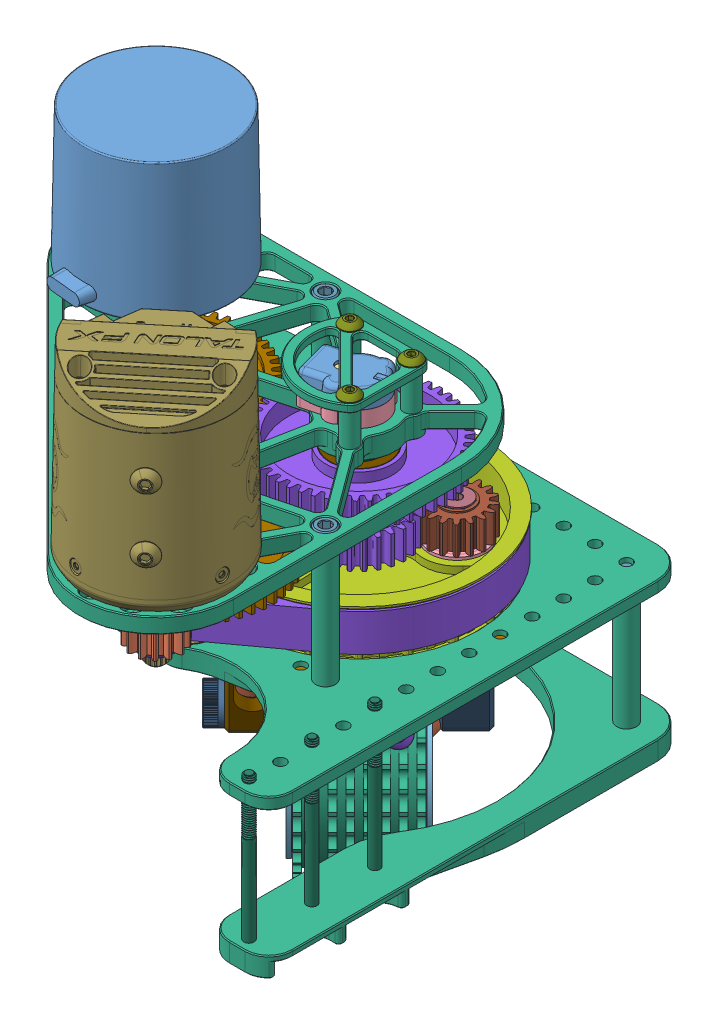
SolidWorks assembly MK4i Swerve Module+KRAKEN, configuration Valor predeterminado. Lengths in mm.
Overall size (247.38 247.71 250.53).
90 component instances, 48 part files, 4 mates.
Components (placement in the parent):
- CANcoder Assembly_MIR1.stp-1: CANcoder Assembly_MIR1.stp [Valor predeterminado] at (-66.675 132.3975 66.675) x (-0.260871 0 -0.965374) z (0 -1 0) size (21.75 26.91 13.51)
  - CANcoder Top Housing_MIR1.stp-1: CANcoder Top Housing_MIR1.stp [Valor predeterminado] at origin size (21.53 26.79 8.94)
  - CANcoder PCA_MIR1.stp-1: CANcoder PCA_MIR1.stp [Valor predeterminado] at (0 0 -22.3055) size (15.93 23.27 3.18)
  - CANcoder Screw_MIR1.stp-1: CANcoder Screw_MIR1.stp [Valor predeterminado] at origin size (4.24 4.24 12.65)
  - CANcoder Bottom Housing_MIR1.stp-1: CANcoder Bottom Housing_MIR1.stp [Valor predeterminado] at origin size (21.75 26.91 6.35)
- MK4 Billet Wheel Assembly_MIR1.stp-1: MK4 Billet Wheel Assembly_MIR1.stp [Valor predeterminado] at (-66.675 50.7435 66.675) x (0.707107 0 -0.707107) z (-0.41117 -0.813559 -0.41117) size (42.28 100.13 100.13)
  - Wheel, SDS, Nitrile Tread, 4in X 1.5in, Bearing Bore_MIR1.stp-1: Wheel, SDS, Nitrile Tread, 4in X 1.5in, Bearing Bore_MIR1.stp [Valor predeterminado] at origin size (42.28 88.9 88.9)
  - Tread, Blue Nitrile 4in X 1.5in_MIR1.stp-1: Tread, Blue Nitrile 4in X 1.5in_MIR1.stp [Valor predeterminado] at origin size (38.1 100.13 100.13)
  - Screw, 10-32 X .75, Button, 91255A269_91255A269_MIR1.stp-1: Screw, 10-32 X .75, Button, 91255A269_91255A269_MIR1.stp [Valor predeterminado] at (-4.826 0 -20.6375) x (0 -0.847203 0.531269) z (1 0 0) size (9.17 9.17 21.62)
  - Screw, 10-32 X .75, Button, 91255A269_91255A269_MIR1.stp-2: Screw, 10-32 X .75, Button, 91255A269_91255A269_MIR1.stp [Valor predeterminado] at (-4.826 -17.8726 -10.3187) x (0 -0.99925 0.038711) z (1 0 0) size (9.17 9.17 21.62)
  - Screw, 10-32 X .75, Button, 91255A269_91255A269_MIR1.stp-3: Screw, 10-32 X .75, Button, 91255A269_91255A269_MIR1.stp [Valor predeterminado] at (-4.826 -17.8726 10.3187) x (0 -0.986188 0.165633) z (1 0 0) size (9.17 9.17 21.62)
  - Screw, 10-32 X .75, Button, 91255A269_91255A269_MIR1.stp-4: Screw, 10-32 X .75, Button, 91255A269_91255A269_MIR1.stp [Valor predeterminado] at (-4.826 0 20.6375) x (0 -0.966455 0.256836) z (1 0 0) size (9.17 9.17 21.62)
  - Screw, 10-32 X .75, Button, 91255A269_91255A269_MIR1.stp-5: Screw, 10-32 X .75, Button, 91255A269_91255A269_MIR1.stp [Valor predeterminado] at (-4.826 17.8726 10.3187) x (0 -0.95104 0.309068) z (1 0 0) size (9.17 9.17 21.62)
  - Screw, 10-32 X .75, Button, 91255A269_91255A269_MIR1.stp-6: Screw, 10-32 X .75, Button, 91255A269_91255A269_MIR1.stp [Valor predeterminado] at (-4.826 17.8726 -10.3187) x (0 -0.947988 0.318305) z (1 0 0) size (9.17 9.17 21.62)
  - Screw, 10-32 X .5, Button, 97763A232_97763A232_MIR1.stp-1: Screw, 10-32 X .5, Button, 97763A232_97763A232_MIR1.stp [Valor predeterminado] at (11.1125 -40.6604 -7.1695) x (-0.785325 0.107503 -0.609678) z (0 0.984808 0.173648) size (9.17 9.17 15.27)
  - Screw, 10-32 X .5, Button, 97763A232_97763A232_MIR1.stp-2: Screw, 10-32 X .5, Button, 97763A232_97763A232_MIR1.stp [Valor predeterminado] at (-11.1125 -40.6604 -7.1695) x (-0.636812 0.133886 -0.759306) z (0 0.984808 0.173648) size (9.17 9.17 15.27)
  - Screw, 10-32 X .5, Button, 97763A232_97763A232_MIR1.stp-3: Screw, 10-32 X .5, Button, 97763A232_97763A232_MIR1.stp [Valor predeterminado] at (-11.1125 -40.6604 7.1695) x (0.726076 -0.119403 -0.677168) z (0 0.984808 -0.173648) size (9.17 9.17 15.27)
  - Screw, 10-32 X .5, Button, 97763A232_97763A232_MIR1.stp-4: Screw, 10-32 X .5, Button, 97763A232_97763A232_MIR1.stp [Valor predeterminado] at (11.1125 -40.6604 7.1695) x (0.841108 -0.09392 -0.53265) z (0 0.984808 -0.173648) size (9.17 9.17 15.27)
  - Screw, 10-32 X .5, Button, 97763A232_97763A232_MIR1.stp-5: Screw, 10-32 X .5, Button, 97763A232_97763A232_MIR1.stp [Valor predeterminado] at (-11.1125 20.6438 35.7562) x (0.804058 -0.514897 0.297276) z (0 -0.5 -0.866025) size (9.17 9.17 15.27)
  - Screw, 10-32 X .5, Button, 97763A232_97763A232_MIR1.stp-6: Screw, 10-32 X .5, Button, 97763A232_97763A232_MIR1.stp [Valor predeterminado] at (11.1125 20.6438 35.7562) x (0.926716 -0.32542 0.187881) z (0 -0.5 -0.866025) size (9.17 9.17 15.27)
  - Screw, 10-32 X .5, Button, 97763A232_97763A232_MIR1.stp-7: Screw, 10-32 X .5, Button, 97763A232_97763A232_MIR1.stp [Valor predeterminado] at (11.1125 20.6438 -35.7562) x (0.200031 0.848523 0.489895) z (0 -0.5 0.866025) size (9.17 9.17 15.27)
  - Screw, 10-32 X .5, Button, 97763A232_97763A232_MIR1.stp-8: Screw, 10-32 X .5, Button, 97763A232_97763A232_MIR1.stp [Valor predeterminado] at (-11.1125 20.6438 -35.7562) x (0.515054 0.74232 0.428579) z (0 -0.5 0.866025) size (9.17 9.17 15.27)
- Screw, 10-32 X .25, Button, 91255A261_91255A261_MIR1.stp-1: Screw, 10-32 X .25, Button, 91255A261_91255A261_MIR1.stp [Valor predeterminado] at (-42.2285 89.5096 114.6539) x (1 0 0) z (0 1 0) size (9.17 9.17 8.92)
- Screw, 10-32 X .25, Button, 91255A261_91255A261_MIR1.stp-2: Screw, 10-32 X .25, Button, 91255A261_91255A261_MIR1.stp [Valor predeterminado] at (-104.7513 89.5096 104.7513) x (0.982082 0 0.188455) z (0 1 0) size (9.17 9.17 8.92)
- Screw, 10-32 X .25, Button, 91255A261_91255A261_MIR1.stp-3: Screw, 10-32 X .25, Button, 91255A261_91255A261_MIR1.stp [Valor predeterminado] at (-114.6539 89.5096 42.2285) x (0.918365 0 0.395734) z (0 1 0) size (9.17 9.17 8.92)
- Screw, 10-32 X .25, Button, 91255A261_91255A261_MIR1.stp-4: Screw, 10-32 X .25, Button, 91255A261_91255A261_MIR1.stp [Valor predeterminado] at (-63.5129 89.5096 12.9199) x (0.8 0 0.6) z (0 1 0) size (9.17 9.17 8.92)
- Screw, 10-32 X .25, Button, 91255A261_91255A261_MIR1.stp-5: Screw, 10-32 X .25, Button, 91255A261_91255A261_MIR1.stp [Valor predeterminado] at (-12.9199 89.5096 63.5129) x (0.63358 0 0.773678) z (0 1 0) size (9.17 9.17 8.92)
- Screw, Shoulder, .375 X 2.5, 5_16-18, 91259A634_91259A634_MIR1.stp-1: Screw, Shoulder, .375 X 2.5, 5_16-18, 91259A634_91259A634_MIR1.stp [Valor predeterminado] at (-93.8403 50.7435 93.8403) x (-0.019195 -0.999631 -0.019195) z (-0.706846 0.027146 -0.706846) size (14.29 82.55 14.29)
- Screw, .25-20 X 1 Socket, 91251A542_91251A542_MIR1.stp-1: Screw, .25-20 X 1 Socket, 91251A542_91251A542_MIR1.stp [Valor predeterminado] at (-102.596 101.6 73.8592) x (0.964329 0 -0.264706) z (0 -1 0) size (9.53 9.53 31.75)
- Screw, .25-20 X 1 Socket, 91251A542_91251A542_MIR1.stp-2: Screw, .25-20 X 1 Socket, 91251A542_91251A542_MIR1.stp [Valor predeterminado] at (-73.8592 101.6 102.596) x (0.982082 0 0.188455) z (0 -1 0) size (9.53 9.53 31.75)
- Screw, .25-20 X .625, 91251A539_91251A539_MIR1.stp-1: Screw, .25-20 X .625, 91251A539_91251A539_MIR1.stp [Valor predeterminado] at (-59.4908 83.2802 30.754) x (1 0 0) z (0 1 0) size (9.53 9.53 22.23)
- Screw, .25-20 X .625, 91251A539_91251A539_MIR1.stp-2: Screw, .25-20 X .625, 91251A539_91251A539_MIR1.stp [Valor predeterminado] at (-30.754 83.2802 59.4908) x (0.982082 0 0.188455) z (0 1 0) size (9.53 9.53 22.23)
- Screw, .25-20 X .625, 91251A539_91251A539_MIR1.stp-3: Screw, .25-20 X .625, 91251A539_91251A539_MIR1.stp [Valor predeterminado] at (-66.675 126.2062 66.675) x (0 0 -1) z (0 -1 0) size (9.53 9.53 22.23)
- Screw, 12-24 X .625, Flat, 91253A282_91253A282_MIR1.stp-1: Screw, 12-24 X .625, Flat, 91253A282_91253A282_MIR1.stp [Valor predeterminado] at (-46.8646 122.8979 46.8646) x (-0.837169 0 0.546944) z (0 -1 0) size (10.72 10.72 15.88)
- Screw, 10-32 X 2.25, 91251A354_91251A354_MIR1.stp-1: Screw, 10-32 X 2.25, 91251A354_91251A354_MIR1.stp [Valor predeterminado] at (-124.5154 92.0115 124.5154) x (-0.750514 0 -0.660855) z (0 1 0) size (7.92 7.92 61.98)
- Screw, 10-32 X 2.25, 91251A354_91251A354_MIR1.stp-2: Screw, 10-32 X 2.25, 91251A354_91251A354_MIR1.stp [Valor predeterminado] at (-32.639 92.0115 114.3) x (-0.612525 0 -0.790452) z (0 1 0) size (7.92 7.92 61.98)
- Screw, 10-32 X 2.25, 91251A354_91251A354_MIR1.stp-3: Screw, 10-32 X 2.25, 91251A354_91251A354_MIR1.stp [Valor predeterminado] at (-114.3 92.0115 32.639) x (-0.427723 0 -0.90391) z (0 1 0) size (7.92 7.92 61.98)
- Screw, 10-32 X 2.25, 91251A354_91251A354_MIR1.stp-4: Screw, 10-32 X 2.25, 91251A354_91251A354_MIR1.stp [Valor predeterminado] at (-12.7 98.4885 12.7) x (0.90391 0 0.427723) z (0 -1 0) size (7.92 7.92 61.98)
- Screw, 8-32 X 2.5, 91251A207_91251A207_MIR1.stp-1: Screw, 8-32 X 2.5, 91251A207_91251A207_MIR1.stp [Valor predeterminado] at (-114.3 102.6795 12.7) x (-0.783238 0 0.621722) z (0 -1 0) size (6.86 6.86 66.17)
- Screw, 8-32 X 2.5, 91251A207_91251A207_MIR1.stp-2: Screw, 8-32 X 2.5, 91251A207_91251A207_MIR1.stp [Valor predeterminado] at (-139.7 102.6795 12.7) x (-0.925243 0 0.379375) z (0 -1 0) size (6.86 6.86 66.17)
- Screw, 8-32 X 2.5, 91251A207_91251A207_MIR1.stp-3: Screw, 8-32 X 2.5, 91251A207_91251A207_MIR1.stp [Valor predeterminado] at (-165.1 102.6795 12.7) x (-0.985271 0 0.170998) z (0 -1 0) size (6.86 6.86 66.17)
- Screw, 8-32 X 2.5, 91251A207_91251A207_MIR1.stp-4: Screw, 8-32 X 2.5, 91251A207_91251A207_MIR1.stp [Valor predeterminado] at (-12.7 102.6795 114.3) x (-0.997902 0 -0.064746) z (0 -1 0) size (6.86 6.86 66.17)
- Screw, 8-32 X 2.5, 91251A207_91251A207_MIR1.stp-5: Screw, 8-32 X 2.5, 91251A207_91251A207_MIR1.stp [Valor predeterminado] at (-12.7 102.6795 139.7) x (-0.953572 0 -0.301166) z (0 -1 0) size (6.86 6.86 66.17)
- Screw, 8-32 X 2.5, 91251A207_91251A207_MIR1.stp-6: Screw, 8-32 X 2.5, 91251A207_91251A207_MIR1.stp [Valor predeterminado] at (-12.7 102.6795 165.1) x (-0.86157 0 -0.507639) z (0 -1 0) size (6.86 6.86 66.17)
- Screw, 8-32 X .875, Button, 91255A166_91255A166_MIR1.stp-1: Screw, 8-32 X .875, Button, 91255A166_91255A166_MIR1.stp [Valor predeterminado] at (-80.9791 172.8661 56.1146) x (1 0 0) z (0 -1 0) size (7.92 7.92 24.45)
- Screw, 8-32 X .875, Button, 91255A166_91255A166_MIR1.stp-2: Screw, 8-32 X .875, Button, 91255A166_91255A166_MIR1.stp [Valor predeterminado] at (-56.1231 172.8661 56.1146) x (0.982082 0 0.188455) z (0 -1 0) size (7.92 7.92 24.45)
- Screw, 8-32 X .875, Button, 91255A166_91255A166_MIR1.stp-3: Screw, 8-32 X .875, Button, 91255A166_91255A166_MIR1.stp [Valor predeterminado] at (-56.1231 172.8661 80.9854) x (0.918365 0 0.395734) z (0 -1 0) size (7.92 7.92 24.45)
- Shim, 8mm ID X 14mm OD X .5mm Thick, 98055A115_98055A115_MIR1.stp-1: Shim, 8mm ID X 14mm OD X .5mm Thick, 98055A115_98055A115_MIR1.stp [Valor predeterminado] at (-46.8646 73.9775 46.8646) x (0.942304 0 0.334759) z (-0.334759 0 0.942304) size (14 1 14)
- Bearing, 6802_MIR1.stp-1: Bearing, 6802_MIR1.stp [Valor predeterminado] at (-66.675 138.5216 66.675) x (0.972423 0 -0.233226) z (0.233226 0 0.972423) size (24 5 24)
- Bearing, 6802_MIR1.stp-2: Bearing, 6802_MIR1.stp [Valor predeterminado] at (-66.675 147.8675 66.675) x (0.877163 0 -0.480193) z (0.480193 0 0.877163) size (24 5 24)
- Bearing, 6802_MIR1.stp-3: Bearing, 6802_MIR1.stp [Valor predeterminado] at (-66.675 118.1216 66.675) x (0.639486 0 -0.768802) z (0.768802 0 0.639486) size (24 5 24)
- Bearing, R6ZZ_MIR1.stp-1: Bearing, R6ZZ_MIR1.stp [Valor predeterminado] at (-79.2721 50.7435 79.2721) x (-0.694824 0.18558 -0.694824) z (-0.131225 -0.982629 -0.131225) size (22.23 7.14 22.23)
- Bearing, R8ZZ_MIR1.stp-1: Bearing, R8ZZ_MIR1.stp [Valor predeterminado] at (-57.5286 50.7435 57.5286) x (-0.158587 -0.974526 -0.158587) z (0.689094 -0.224275 0.689094) size (35.76 21.72 36.1)
- Bearing, 688_MIR1.stp-1: Bearing, 688_MIR1.stp [Valor predeterminado] at (-46.8646 71.4775 46.8646) x (0 -1 0) z (0.336154 0 0.941807) size (5 16 16)
- Bearing, .375 ThunderHex, Flanged, 217-5829_MIR1.stp-1: Bearing, .375 ThunderHex, Flanged, 217-5829_MIR1.stp [Valor predeterminado] at (-46.8646 102.3938 46.8646) x (0.903016 0 -0.429606) z (0.429606 0 0.903016) size (24.51 7.14 24.51)
- Bevel Gear, 1545_MIR1.stp-1: Bevel Gear, 1545_MIR1.stp [Valor predeterminado] at (-46.8646 84.4935 46.8646) x (-0.830686 0 0.556741) z (0.556741 0 0.830686) size (133.56 133.56 133.56)
- Bearing, 688_MIR1.stp-2: Bearing, 688_MIR1.stp [Valor predeterminado] at (-128.0498 97.5125 83.2602) x (0 -1 0) z (0.444562 0 0.895748) size (5 16 16)
- Bearing, R188ZZ, 217-3489_MIR1.stp-1: Bearing, R188ZZ, 217-3489_MIR1.stp [Valor predeterminado] at (-77.6314 97.6313 123.9376) x (-0.188457 0 0.982081) z (-0.982081 0 -0.188457) size (12.7 4.76 12.7)
- Bearing, 688_MIR1.stp-3: Bearing, 688_MIR1.stp [Valor predeterminado] at (-77.6314 150.1375 123.9376) x (0 -1 0) z (0.336154 0 0.941807) size (5 16 16)
- Bearing, 688_MIR1.stp-4: Bearing, 688_MIR1.stp [Valor predeterminado] at (-128.0498 148.8167 83.2602) x (0 -1 0) z (0.336154 0 0.941807) size (5 16 16)
- Bearing, A035XPO_SA035XPO_MIR1.stp-1: Bearing, A035XPO_SA035XPO_MIR1.stp [Valor predeterminado] at (-66.675 95.25 66.675) x (0.978935 0 -0.20417) z (0.20417 0 0.978935) size (101.6 6.35 101.6)
- Double Gear, 20DP, 28T, 50T_MIR1.stp-1: Double Gear, 20DP, 28T, 50T_MIR1.stp [Valor predeterminado] at (-66.675 110.1225 66.675) x (-0.730582 0 0.682825) z (0 -1 0) size (65.97 66.04 34.49)
- Gear, 50T, 20DP, .375Hex_MIR1.stp-1: Gear, 50T, 20DP, .375Hex_MIR1.stp [Valor predeterminado] at (-128.0498 139.8651 83.2602) x (0.985885 0 0.167422) z (0 -1 0) size (65.97 66.04 12.65)
- Gear, 50T, 20DP, .375Hex_MIR1.stp-2: Gear, 50T, 20DP, .375Hex_MIR1.stp [Valor predeterminado] at (-77.6314 128.4859 123.9376) x (-0.963721 0 -0.266911) z (0 -1 0) size (65.97 66.04 12.65)
- Bevel Gear, 4515_MIR1.stp-1: Bevel Gear, 4515_MIR1.stp [Valor predeterminado] at (-54.7746 50.7435 54.7746) x (0.575273 -0.581482 0.575273) z (0.41117 0.813559 0.41117) size (68.39 7.78 68.43)
- Gear, 17T, 20DP, .375Hex_MIR1.stp-1: Gear, 17T, 20DP, .375Hex_MIR1.stp [Valor predeterminado] at (-46.8646 115.8367 46.8646) x (0 1 0) z (-0.115868 0 -0.993265) size (12.6 23.99 24.09)
- MK4i Steering Shaft Tall_MIR1.stp-1: MK4i Steering Shaft Tall_MIR1.stp [Valor predeterminado] at (-77.6314 152.5105 123.9376) x (0.998641 0 0.05212) z (-0.05212 0 0.998641) size (17.78 57.04 17.78)
- MK4i Steering Shaft Spacer_MIR1.stp-1: MK4i Steering Shaft Spacer_MIR1.stp [Valor predeterminado] at (-77.6314 134.8105 123.9376) x (-0.728275 0 0.685285) z (-0.685285 0 -0.728275) size (13.36 12.7 13.36)
- MK4 Intermediate Shaft_MIR1.stp-1: MK4 Intermediate Shaft_MIR1.stp [Valor predeterminado] at (-46.8646 68.3577 46.8646) x (0.999953 0 -0.009669) z (0.009669 0 0.999953) size (11.68 51.44 11.68)
- MK3 Center Column_MIR1.stp-1: MK3 Center Column_MIR1.stp [Valor predeterminado] at (-66.675 113.0816 66.675) x (-0.707107 0 -0.707107) z (0.707107 0 -0.707107) size (17.27 40.32 17.27)
- MK4i Shaft, Drive Idler_MIR1.stp-1: MK4i Shaft, Drive Idler_MIR1.stp [Valor predeterminado] at (-128.0498 100.0125 83.2602) size (13.36 56.18 13.36)
- Screw, 3-48 X .1875, Pan Phillips, 90272A091_90272A091_MIR1.stp-1: Screw, 3-48 X .1875, Pan Phillips, 90272A091_90272A091_MIR1.stp [Valor predeterminado] at (-68.5859 150.495 73.8677) x (1 0 0) z (0 -1 0) size (4.9 4.9 6.49)
- Screw, 3-48 X .1875, Pan Phillips, 90272A091_90272A091_MIR1.stp-2: Screw, 3-48 X .1875, Pan Phillips, 90272A091_90272A091_MIR1.stp [Valor predeterminado] at (-64.7641 150.495 59.4823) x (0.911631 0 0.411009) z (0 -1 0) size (4.9 4.9 6.49)
- magnet_MIR1.stp-1: magnet_MIR1.stp [Valor predeterminado] at (-66.675 140.7033 66.675) x (-0.536649 0 0.843806) z (-0.843806 0 -0.536649) size (6.35 12.7 6.35)
- Motor, NEO_MIR1.stp-1: Motor, NEO_MIR1.stp [Valor predeterminado] at (-158.75 153.9875 56.515) x (-0.647262 0 -0.762267) z (0 1 0) size (59.98 59.98 90)
- Shim, 8mm ID X 14mm OD X .5mm Thick, 98055A115_98055A115_MIR1.stp-2: Shim, 8mm ID X 14mm OD X .5mm Thick, 98055A115_98055A115_MIR1.stp [Valor predeterminado] at (-56.515 122.5625 158.75) x (0.942304 0 0.334759) z (-0.334759 0 0.942304) size (14 1 14)
- Gear, 20DP, 14T, 8mm REV1_MIR1.stp-1: Gear, 20DP, 14T, 8mm REV1_MIR1.stp [Valor predeterminado] at (-56.515 123.5625 158.75) x (0 1 0) z (0.866025 0 -0.5) size (12.7 19.97 20.32)
- Retaining Ring, 8mm, 98430A132_98430A132_MIR1.stp-1: Retaining Ring, 8mm, 98430A132_98430A132_MIR1.stp [Valor predeterminado] at (-56.515 136.2625 158.75) x (0 1 0) z (0.12503 0 0.992153) size (1.07 14.83 14.83)
- Gear, 20DP, 14T, 8mm REV1_MIR1.stp-2: Gear, 20DP, 14T, 8mm REV1_MIR1.stp [Valor predeterminado] at (-158.75 133.675 56.515) x (0 1 0) z (0.866025 0 0.5) size (12.7 19.97 20.32)
- Spacer, 8mmID X .437 OD X 0.437 L_MIR1.stp-1: Spacer, 8mmID X .437 OD X 0.437 L_MIR1.stp [Valor predeterminado] at (-158.75 122.5625 56.515) size (11.11 11.11 11.11)
- Retaining Ring, 8mm, 98430A132_98430A132_MIR1.stp-2: Retaining Ring, 8mm, 98430A132_98430A132_MIR1.stp [Valor predeterminado] at (-158.75 146.375 56.515) x (0 1 0) z (-0.064186 0 0.997938) size (1.07 14.83 14.83)
- Machine Key, 2 X 2 X 12mm_MIR1.stp-1: Machine Key, 2 X 2 X 12mm_MIR1.stp [Valor predeterminado] at (-160.675 140.025 59.8492) x (-0.866025 0 -0.5) z (0.5 0 -0.866025) size (2 12 2)
- Machine Key, 2 X 2 X 12mm_MIR1.stp-2: Machine Key, 2 X 2 X 12mm_MIR1.stp [Valor predeterminado] at (-54.59 129.9125 162.0842) x (0.866025 0 -0.5) z (0.5 0 0.866025) size (2 12 2)
- MK4i Master Part_NEO Config_MIR1.stp-1: MK4i Master Part_NEO Config_MIR1.stp [Valor predeterminado] at origin size (189.87 134.14 189.87)
- MK3 Base Pulley Tall_MIR1.stp-1: MK3 Base Pulley Tall_MIR1.stp [Valor predeterminado] at (-66.675 98.425 66.675) x (-0.707107 0 -0.707107) z (0.707107 0 -0.707107) size (98.42 27.08 98.42)
- Belt, 320-5M-15_MIR1.stp-1: Belt, 320-5M-15_MIR1.stp [Valor predeterminado] at (-66.675 109.752 66.675) x (0.982183 0 0.187927) z (-0.187927 0 0.982183) size (97.78 15 116.29)
- Wheel Mount A_MIR1.stp-1: Wheel Mount A_MIR1.stp [Valor predeterminado] at (-88.2276 50.7435 88.2276) x (-0.707107 0 0.707107) z (-0.707107 0 -0.707107) size (17.09 49.74 57.15)
- Wheel Mount B Gen2_MIR1.stp-1: Wheel Mount B Gen2_MIR1.stp [Valor predeterminado] at (-45.1224 50.7435 45.1224) x (-0.707107 0 0.707107) z (-0.707107 0 -0.707107) size (15.88 49.27 57.15)
- MK4 Wheel Spacer_MIR1.stp-1: MK4 Wheel Spacer_MIR1.stp [Valor predeterminado] at (-76.7015 50.7435 76.7015) x (-0.707107 0 0.707107) z (-0.522819 0.67329 -0.522819) size (36.72 15.11 15.11)
- KRAKEN-1: KRAKEN [Valor predeterminado] at (-56.515 185.2285 158.75) x (0.772689 0 -0.634785) z (0 -1 0) size (65.83 65.88 111.99)
Mates (geometry in assembly coordinates):
- Concêntrico1: concentric anti-aligned: cylinder of Motor, NEO_MIR1.stp-1 through (-158.75 150.4875 56.515) axis (0 -1 0) radius 9.525; cylinder of MK4i Master Part_NEO Config_MIR1.stp-1 through (-158.75 153.9875 56.515) axis (0 1 0) radius 9.5631
- Coincidente1: coincident anti-aligned: plane of Motor, NEO_MIR1.stp-1 through (-158.75 153.9875 56.515) normal (0 -1 0); plane of MK4i Master Part_NEO Config_MIR1.stp-1 through (-56.515 153.9875 158.75) normal (0 1 0)
- Concêntrico2: concentric aligned: cylinder of MK4i Master Part_NEO Config_MIR1.stp-1 through (-56.515 153.9875 158.75) axis (0 1 0) radius 9.5631; cylinder of KRAKEN-1 through (-56.515 185.2285 158.75) axis (0 1 0) radius 9.525
- Coincidente2: coincident anti-aligned: plane of MK4i Master Part_NEO Config_MIR1.stp-1 through (-56.515 153.9875 158.75) normal (0 1 0); plane of KRAKEN-1 through (-56.515 153.9875 158.75) normal (0 -1 0)
